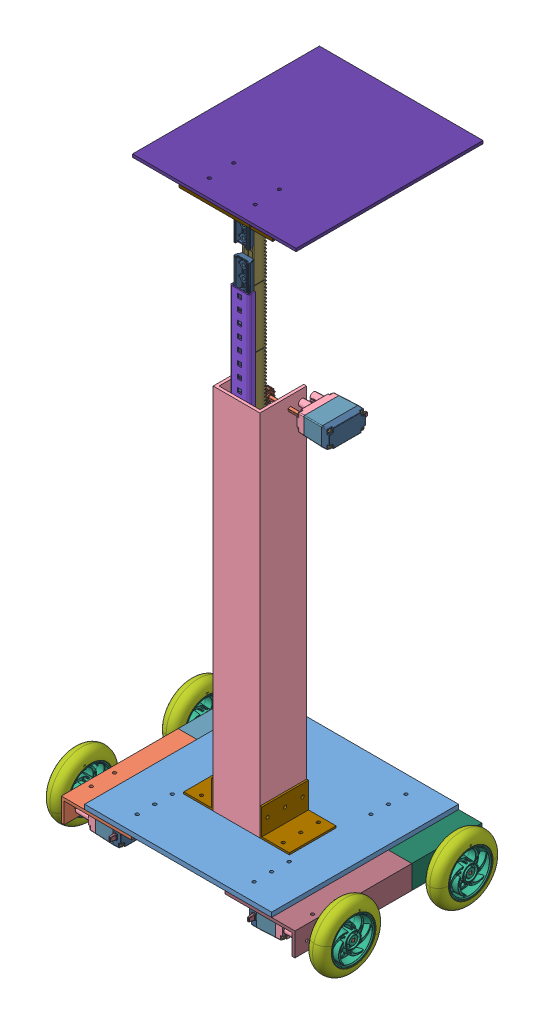
SolidWorks assembly mte380_Assy_01_lift_03., configuration Default. Lengths in mm.
Overall size (307.05 662.06 247.45).
139 component instances, 39 part files, 97 mates.
Components (placement in the parent):
- mte380_01_lift_base_02-1: mte380_01_lift_base_02 [Default] at (94.2351 110.2702 143.398) size (203.2 5 203.2)
- mte380_01_motor_bot_L_bracket_01-1: mte380_01_motor_bot_L_bracket_01 [Default] at (43.4351 110.2702 168.798) size (76.2 25.4 127)
- mte380_Assy_motor_vex_393_01-1: mte380_Assy_motor_vex_393_01 [Default] at (16.7501 95.0302 218.0279) x (0 0 -1) z (1 0 0) size (277.81 20.59 51.81)
  - SPPM206-0150BO-1: SPPM206-0150BO [Default] at (17.3 7.3 -1.5) x (1 0 0) z (0 -1 0) size (3.3 16.36 3.3)
  - 276-2181-003 Rev1-1: 276-2181-003 Rev1 [Default] at (0 0 -28) size (38.95 18.95 25.5)
  - 276-2177-019 Rev1-1: 276-2177-019 Rev1 [Default] at (-14.2702 0 -28) x (0.144195 -0.989549 0) z (0.989549 0.144195 0) size (6.3 15.8 6.3)
  - 276-2181-011 Rev1-1: 276-2181-011 Rev1 [Default] at (11.1298 0 -11) x (-1 0 0) z (0 1 0) size (11 4 11)
  - 276-2177-017 Rev1-1: 276-2177-017 Rev1 [Default] at (-245.51 0.1 2.5) size (248.21 15.59 2.54) (hidden)
  - QFK-N30QAV-16068-1: QFK-N30QAV-16068 [Default] at (-12.9 0 -23) x (0 1 0) z (0 0 1) size (12 10 26.1)
  - SPPM143-0030BO-1: SPPM143-0030BO [Default] at (-12.9 4.25 -6) x (-1 0 0) z (0 1 0) size (2.4 6.08 2.4)
  - 276-2181-010 Rev1-1: 276-2181-010 Rev1 [Default] at (10.8763 0 -9.4) x (0.878827 0.47714 0) z (0 0 1) size (1.5 1.5 16)
  - 276-2181-001 Rev1-1: 276-2181-001 Rev1 [Default] at origin size (40 20 8.01)
  - 276-2181-006 Rev1-1: 276-2181-006 Rev1 [Default] at (10.8763 0 -1.05) x (-0.259931 -0.965627 0) z (0 0 1) size (14.22 14.25 6.9)
  - 276-2181-007 Rev1-1: 276-2181-007 Rev1 [Default] at (2.1533 -1.4937 -4.4) x (-0.202497 0.979283 0) z (0 0 1) size (14.22 14.25 14.9)
  - 276-2181-010 Rev1-2: 276-2181-010 Rev1 [Default] at (-5.7003 2.586 -9.4) size (1.5 1.5 16)
  - 276-2177-018 Rev1-1: 276-2177-018 Rev1 [Default] at (-18.5 0.1 2.5) x (0 1 0) z (1 0 0) size (6.82 4.47 8.9)
  - 276-2181-006 Rev1-2: 276-2181-006 Rev1 [Default] at (2.1533 -1.4937 2.75) x (-0.071378 0.997449 0) z (0 0 1) size (14.22 14.25 6.9)
  - 276-2181-002 Rev1-1: 276-2181-002 Rev1 [Default] at (0 0 -20) size (40 20 23)
  - 276-2181-009 Rev1-1: 276-2181-009 Rev1 [Default] at (2.1533 -1.4937 -26.5) size (1.5 1.5 33)
  - SPPM206-0150BO-2: SPPM206-0150BO [Default] at (-16.9263 6.9263 -18.5) x (-0.075705 0.99713 0) z (-0.99713 -0.075705 0) size (3.3 16.36 3.3)
  - 276-2181-011 Rev1-2: 276-2181-011 Rev1 [Default] at (11.1298 0 -24) x (-0.997622 -0.068917 0) z (-0.068917 0.997622 0) size (11 4 11)
  - 276-2177-019 Rev1-2: 276-2177-019 Rev1 [Default] at (-1.5702 0 -28) x (0.32391 -0.946088 0) z (0.946088 0.32391 0) size (6.3 15.8 6.3)
  - SPPM206-0150BO-3: SPPM206-0150BO [Default] at (-17.3 -7.3 -1.5) x (0.292947 -0.956129 0) z (-0.956129 -0.292947 0) size (3.3 16.36 3.3)
  - SPPM206-0150BO-4: SPPM206-0150BO [Default] at (16.9263 -6.9263 -18.5) x (0.149257 -0.988799 0) z (0.988799 0.149257 0) size (3.3 16.36 3.3)
  - SPPM206-0150BO-5: SPPM206-0150BO [Default] at (17.3 -7.3 -1.5) x (1 0 0) z (0 -1 0) size (3.3 16.36 3.3)
  - SPPM206-0150BO-6: SPPM206-0150BO [Default] at (-16.9263 -6.9263 -18.5) x (-0.049887 0.998755 0) z (-0.998755 -0.049887 0) size (3.3 16.36 3.3)
  - SPPM206-0150BO-7: SPPM206-0150BO [Default] at (-17.3 7.3 -1.5) x (-0.963198 0.268794 0) z (0.268794 0.963198 0) size (3.3 16.36 3.3)
  - SPPM206-0150BO-8: SPPM206-0150BO [Default] at (16.9263 6.9263 -18.5) x (0.906825 0.421508 0) z (-0.421508 0.906825 0) size (3.3 16.36 3.3)
  - SPPM143-0030BO-2: SPPM143-0030BO [Default] at (-12.9 -4.25 -6) x (-0.988208 -0.153116 0) z (-0.153116 0.988208 0) size (2.4 6.08 2.4)
  - 276-2181-004 Rev1-1: 276-2181-004 Rev1 [Default] at (-12.9 0 -0.1) x (0.94341 -0.331628 0) z (0 0 -1) size (5.17 5.4 3)
  - 276-2181-005 Rev1-1: 276-2181-005 Rev1 [Default] at (-5.7003 2.586 -0.05) x (0.460478 -0.887671 0) z (0 0 1) size (11.88 11.88 5.9)
  - 276-2181-008 Rev1_276-2181-008g-1: 276-2181-008 Rev1_276-2181-008g [Default] at (11.1298 0 -14.5) x (0.267616 -0.963526 0) z (0 0 -1) size (13.83 13.88 17.3)
  - 276-2181-012 Rev1-1: 276-2181-012 Rev1 [Default] at (-12.9 0 -24) size (13.6 13 1)
- mte380_01_vex_shaft_2-1: mte380_01_vex_shaft_2 [Default] at (-31.9499 95.0479 206.9293) x (0 -0.267616 0.963526) z (-1 0 0) size (4.18 4.18 51.01)
- mte380_01_vex_bearing_block-1: mte380_01_vex_bearing_block [Default] at (-24.8662 107.0952 130.6495) x (0 0 -1) z (0 -1 0) size (35.56 10.16 13.39)
- mte380_01_center_shaft_01-1: mte380_01_center_shaft_01 [Default] at (68.8351 115.2702 130.698) size (50.8 400 50.8)
- mte380_Assy_wheel_vex_275-1: mte380_Assy_wheel_vex_275 [Default] at (-45.4869 83.9602 188.1506) x (0 0.267616 -0.963526) z (1 0 0) size (69.86 69.86 20.66)
  - SMALL-WHEEL-RIM-1: SMALL-WHEEL-RIM [Default] at (-15.1515 15.6838 -2.6601) size (61.43 61.43 9.24)
  - SMALL-WHEEL-HUB-1: SMALL-WHEEL-HUB [Default] at (-15.1515 15.6838 -2.6601) size (61.36 61.43 20.66)
  - SMALL-WHEEL-TIRE-1: SMALL-WHEEL-TIRE [Default] at (-15.1515 15.6838 -2.6601) x (1 0 0) z (0 -1 0) size (69.86 19.99 69.86)
- mte380_01_vex_rack_guide-1: mte380_01_vex_rack_guide [Default] at (94.2351 324.7702 178.323) x (-1 0 0) z (0 0 -1) size (20.84 444.5 8.8)
- mte380_01_vert_rack_bracket_01-1: mte380_01_vert_rack_bracket_01 [Default] at (119.6351 145.2702 130.698) size (32 30 50.8)
- mte380_01_vert_rack_bracket_01-2: mte380_01_vert_rack_bracket_01 [Default] at (68.8351 145.2702 181.498) x (-1 0 0) z (0 0 -1) size (32 30 50.8)
- mte380_01_vex_rack_slide-1: mte380_01_vex_rack_slide [Default] at (94.2351 619.0732 173.3216) x (1 0 0) z (0 1 0) size (17.45 8.37 50.79)
- mte380_01_vex_pinion_12-1: mte380_01_vex_pinion_12 [Default] at (93.6302 502.9979 149.2208) x (0 0.267616 -0.963526) z (1 0 0) size (14.8 14.8 9.53)
- mte380_01_vex_rack-1: mte380_01_vex_rack [Default] at (94.2351 650.8232 168.7501) x (0 1 0) z (-1 0 0) size (63 14.6 12.7)
- mte380_01_vex_rack_slide-2: mte380_01_vex_rack_slide [Default] at (94.2351 682.5732 173.3216) x (1 0 0) z (0 1 0) size (17.45 8.37 50.79)
- mte380_01_motor_bot_R_bracket_01-1: mte380_01_motor_bot_R_bracket_01 [Default] at (145.0351 110.2702 244.998) x (-1 0 0) z (0 0 -1) size (76.2 25.4 127)
- mte380_Assy_motor_vex_393_01-2: mte380_Assy_motor_vex_393_01 [Default] at (172.3201 95.0302 218.0279) x (0 0 -1) z (-1 0 0) size (277.81 20.59 51.81)
  - SPPM206-0150BO-1: SPPM206-0150BO [Default] at (17.3 7.3 -1.5) x (1 0 0) z (0 -1 0) size (3.3 16.36 3.3)
  - 276-2181-003 Rev1-1: 276-2181-003 Rev1 [Default] at (0 0 -28) size (38.95 18.95 25.5)
  - 276-2177-019 Rev1-1: 276-2177-019 Rev1 [Default] at (-14.2702 0 -28) x (0.144195 -0.989549 0) z (0.989549 0.144195 0) size (6.3 15.8 6.3)
  - 276-2181-011 Rev1-1: 276-2181-011 Rev1 [Default] at (11.1298 0 -11) x (-1 0 0) z (0 1 0) size (11 4 11)
  - 276-2177-017 Rev1-1: 276-2177-017 Rev1 [Default] at (-245.51 0.1 2.5) size (248.21 15.59 2.54) (hidden)
  - QFK-N30QAV-16068-1: QFK-N30QAV-16068 [Default] at (-12.9 0 -23) x (0 1 0) z (0 0 1) size (12 10 26.1)
  - SPPM143-0030BO-1: SPPM143-0030BO [Default] at (-12.9 4.25 -6) x (-1 0 0) z (0 1 0) size (2.4 6.08 2.4)
  - 276-2181-010 Rev1-1: 276-2181-010 Rev1 [Default] at (10.8763 0 -9.4) x (0.878827 0.47714 0) z (0 0 1) size (1.5 1.5 16)
  - 276-2181-001 Rev1-1: 276-2181-001 Rev1 [Default] at origin size (40 20 8.01)
  - 276-2181-006 Rev1-1: 276-2181-006 Rev1 [Default] at (10.8763 0 -1.05) x (-0.259931 -0.965627 0) z (0 0 1) size (14.22 14.25 6.9)
  - 276-2181-007 Rev1-1: 276-2181-007 Rev1 [Default] at (2.1533 -1.4937 -4.4) x (-0.202497 0.979283 0) z (0 0 1) size (14.22 14.25 14.9)
  - 276-2181-010 Rev1-2: 276-2181-010 Rev1 [Default] at (-5.7003 2.586 -9.4) size (1.5 1.5 16)
  - 276-2177-018 Rev1-1: 276-2177-018 Rev1 [Default] at (-18.5 0.1 2.5) x (0 1 0) z (1 0 0) size (6.82 4.47 8.9)
  - 276-2181-006 Rev1-2: 276-2181-006 Rev1 [Default] at (2.1533 -1.4937 2.75) x (-0.071378 0.997449 0) z (0 0 1) size (14.22 14.25 6.9)
  - 276-2181-002 Rev1-1: 276-2181-002 Rev1 [Default] at (0 0 -20) size (40 20 23)
  - 276-2181-009 Rev1-1: 276-2181-009 Rev1 [Default] at (2.1533 -1.4937 -26.5) size (1.5 1.5 33)
  - SPPM206-0150BO-2: SPPM206-0150BO [Default] at (-16.9263 6.9263 -18.5) x (-0.075705 0.99713 0) z (-0.99713 -0.075705 0) size (3.3 16.36 3.3)
  - 276-2181-011 Rev1-2: 276-2181-011 Rev1 [Default] at (11.1298 0 -24) x (-0.997622 -0.068917 0) z (-0.068917 0.997622 0) size (11 4 11)
  - 276-2177-019 Rev1-2: 276-2177-019 Rev1 [Default] at (-1.5702 0 -28) x (0.32391 -0.946088 0) z (0.946088 0.32391 0) size (6.3 15.8 6.3)
  - SPPM206-0150BO-3: SPPM206-0150BO [Default] at (-17.3 -7.3 -1.5) x (0.292947 -0.956129 0) z (-0.956129 -0.292947 0) size (3.3 16.36 3.3)
  - SPPM206-0150BO-4: SPPM206-0150BO [Default] at (16.9263 -6.9263 -18.5) x (0.149257 -0.988799 0) z (0.988799 0.149257 0) size (3.3 16.36 3.3)
  - SPPM206-0150BO-5: SPPM206-0150BO [Default] at (17.3 -7.3 -1.5) x (1 0 0) z (0 -1 0) size (3.3 16.36 3.3)
  - SPPM206-0150BO-6: SPPM206-0150BO [Default] at (-16.9263 -6.9263 -18.5) x (-0.049887 0.998755 0) z (-0.998755 -0.049887 0) size (3.3 16.36 3.3)
  - SPPM206-0150BO-7: SPPM206-0150BO [Default] at (-17.3 7.3 -1.5) x (-0.963198 0.268794 0) z (0.268794 0.963198 0) size (3.3 16.36 3.3)
  - SPPM206-0150BO-8: SPPM206-0150BO [Default] at (16.9263 6.9263 -18.5) x (0.906825 0.421508 0) z (-0.421508 0.906825 0) size (3.3 16.36 3.3)
  - SPPM143-0030BO-2: SPPM143-0030BO [Default] at (-12.9 -4.25 -6) x (-0.988208 -0.153116 0) z (-0.153116 0.988208 0) size (2.4 6.08 2.4)
  - 276-2181-004 Rev1-1: 276-2181-004 Rev1 [Default] at (-12.9 0 -0.1) x (0.94341 -0.331628 0) z (0 0 -1) size (5.17 5.4 3)
  - 276-2181-005 Rev1-1: 276-2181-005 Rev1 [Default] at (-5.7003 2.586 -0.05) x (0.460478 -0.887671 0) z (0 0 1) size (11.88 11.88 5.9)
  - 276-2181-008 Rev1_276-2181-008g-1: 276-2181-008 Rev1_276-2181-008g [Default] at (11.1298 0 -14.5) x (0.267616 -0.963526 0) z (0 0 -1) size (13.83 13.88 17.3)
  - 276-2181-012 Rev1-1: 276-2181-012 Rev1 [Default] at (-12.9 0 -24) size (13.6 13 1)
- mte380_01_vex_shaft_2-2: mte380_01_vex_shaft_2 [Default] at (221.0201 95.0615 206.9157) x (0 0.267616 0.963526) z (-1 0 0) size (4.18 4.18 51.01)
- mte380_Assy_wheel_vex_275-4: mte380_Assy_wheel_vex_275 [Default] at (239.8772 75.9124 196.4833) x (0 -0.267616 -0.963526) z (1 0 0) size (69.86 69.86 20.66)
  - SMALL-WHEEL-RIM-1: SMALL-WHEEL-RIM [Default] at (-15.1515 15.6838 -2.6601) size (61.43 61.43 9.24)
  - SMALL-WHEEL-HUB-1: SMALL-WHEEL-HUB [Default] at (-15.1515 15.6838 -2.6601) size (61.36 61.43 20.66)
  - SMALL-WHEEL-TIRE-1: SMALL-WHEEL-TIRE [Default] at (-15.1515 15.6838 -2.6601) x (1 0 0) z (0 -1 0) size (69.86 19.99 69.86)
- mte380_01_vex_shaft_2-3: mte380_01_vex_shaft_2 [Default] at (221.2351 95.0937 79.8345) x (0 0 1) z (-1 0 0) size (4.18 4.18 51.01)
- mte380_01_vex_shaft_2-4: mte380_01_vex_shaft_2 [Default] at (-32.7649 95.1912 79.8345) x (0 0 1) z (-1 0 0) size (4.18 4.18 51.01)
- mte380_01_front_bot_L_bracket_01-1: mte380_01_front_bot_L_bracket_01 [Default] at (43.4351 110.2702 41.798) size (76.2 25.4 76.2)
- mte380_01_front_bot_R_bracket_01-1: mte380_01_front_bot_R_bracket_01 [Default] at (145.0351 110.2702 117.998) x (-1 0 0) z (0 0 -1) size (76.2 25.4 76.2)
- mte380_01_vex_flat_bearing-2: mte380_01_vex_flat_bearing [Default] at (129.0839 107.7302 106.314) x (1 0 0) z (0 1 0) size (7.04 35.56 10.16)
- mte380_01_vex_flat_bearing-3: mte380_01_vex_flat_bearing [Default] at (59.3863 107.7302 53.482) x (-1 0 0) z (0 1 0) size (7.04 35.56 10.16)
- mte380_Assy_wheel_vex_275-5: mte380_Assy_wheel_vex_275 [Default] at (-46.3019 79.4824 64.708) x (0 0 -1) z (1 0 0) size (69.86 69.86 20.66)
  - SMALL-WHEEL-RIM-1: SMALL-WHEEL-RIM [Default] at (-15.1515 15.6838 -2.6601) size (61.43 61.43 9.24)
  - SMALL-WHEEL-HUB-1: SMALL-WHEEL-HUB [Default] at (-15.1515 15.6838 -2.6601) size (61.36 61.43 20.66)
  - SMALL-WHEEL-TIRE-1: SMALL-WHEEL-TIRE [Default] at (-15.1515 15.6838 -2.6601) x (1 0 0) z (0 -1 0) size (69.86 19.99 69.86)
- mte380_Assy_wheel_vex_275-6: mte380_Assy_wheel_vex_275 [Default] at (240.0922 79.4349 64.658) x (0 0 -1) z (1 0 0) size (69.86 69.86 20.66)
  - SMALL-WHEEL-RIM-1: SMALL-WHEEL-RIM [Default] at (-15.1515 15.6838 -2.6601) size (61.43 61.43 9.24)
  - SMALL-WHEEL-HUB-1: SMALL-WHEEL-HUB [Default] at (-15.1515 15.6838 -2.6601) size (61.36 61.43 20.66)
  - SMALL-WHEEL-TIRE-1: SMALL-WHEEL-TIRE [Default] at (-15.1515 15.6838 -2.6601) x (1 0 0) z (0 -1 0) size (69.86 19.99 69.86)
- mte380_Assy_motor_vex_393_01-3: mte380_Assy_motor_vex_393_01 [Default] at (163.3228 503.011 138.0423) x (0 0 1) z (1 0 0) size (277.81 20.59 51.81)
  - SPPM206-0150BO-1: SPPM206-0150BO [Default] at (17.3 7.3 -1.5) x (1 0 0) z (0 -1 0) size (3.3 16.36 3.3)
  - 276-2181-003 Rev1-1: 276-2181-003 Rev1 [Default] at (0 0 -28) size (38.95 18.95 25.5)
  - 276-2177-019 Rev1-1: 276-2177-019 Rev1 [Default] at (-14.2702 0 -28) x (0.144195 -0.989549 0) z (0.989549 0.144195 0) size (6.3 15.8 6.3)
  - 276-2181-011 Rev1-1: 276-2181-011 Rev1 [Default] at (11.1298 0 -11) x (-1 0 0) z (0 1 0) size (11 4 11)
  - 276-2177-017 Rev1-1: 276-2177-017 Rev1 [Default] at (-245.51 0.1 2.5) size (248.21 15.59 2.54) (hidden)
  - QFK-N30QAV-16068-1: QFK-N30QAV-16068 [Default] at (-12.9 0 -23) x (0 1 0) z (0 0 1) size (12 10 26.1)
  - SPPM143-0030BO-1: SPPM143-0030BO [Default] at (-12.9 4.25 -6) x (-1 0 0) z (0 1 0) size (2.4 6.08 2.4)
  - 276-2181-010 Rev1-1: 276-2181-010 Rev1 [Default] at (10.8763 0 -9.4) x (0.878827 0.47714 0) z (0 0 1) size (1.5 1.5 16)
  - 276-2181-001 Rev1-1: 276-2181-001 Rev1 [Default] at origin size (40 20 8.01)
  - 276-2181-006 Rev1-1: 276-2181-006 Rev1 [Default] at (10.8763 0 -1.05) x (-0.259931 -0.965627 0) z (0 0 1) size (14.22 14.25 6.9)
  - 276-2181-007 Rev1-1: 276-2181-007 Rev1 [Default] at (2.1533 -1.4937 -4.4) x (-0.202497 0.979283 0) z (0 0 1) size (14.22 14.25 14.9)
  - 276-2181-010 Rev1-2: 276-2181-010 Rev1 [Default] at (-5.7003 2.586 -9.4) size (1.5 1.5 16)
  - 276-2177-018 Rev1-1: 276-2177-018 Rev1 [Default] at (-18.5 0.1 2.5) x (0 1 0) z (1 0 0) size (6.82 4.47 8.9)
  - 276-2181-006 Rev1-2: 276-2181-006 Rev1 [Default] at (2.1533 -1.4937 2.75) x (-0.071378 0.997449 0) z (0 0 1) size (14.22 14.25 6.9)
  - 276-2181-002 Rev1-1: 276-2181-002 Rev1 [Default] at (0 0 -20) size (40 20 23)
  - 276-2181-009 Rev1-1: 276-2181-009 Rev1 [Default] at (2.1533 -1.4937 -26.5) size (1.5 1.5 33)
  - SPPM206-0150BO-2: SPPM206-0150BO [Default] at (-16.9263 6.9263 -18.5) x (-0.075705 0.99713 0) z (-0.99713 -0.075705 0) size (3.3 16.36 3.3)
  - 276-2181-011 Rev1-2: 276-2181-011 Rev1 [Default] at (11.1298 0 -24) x (-0.997622 -0.068917 0) z (-0.068917 0.997622 0) size (11 4 11)
  - 276-2177-019 Rev1-2: 276-2177-019 Rev1 [Default] at (-1.5702 0 -28) x (0.32391 -0.946088 0) z (0.946088 0.32391 0) size (6.3 15.8 6.3)
  - SPPM206-0150BO-3: SPPM206-0150BO [Default] at (-17.3 -7.3 -1.5) x (0.292947 -0.956129 0) z (-0.956129 -0.292947 0) size (3.3 16.36 3.3)
  - SPPM206-0150BO-4: SPPM206-0150BO [Default] at (16.9263 -6.9263 -18.5) x (0.149257 -0.988799 0) z (0.988799 0.149257 0) size (3.3 16.36 3.3)
  - SPPM206-0150BO-5: SPPM206-0150BO [Default] at (17.3 -7.3 -1.5) x (1 0 0) z (0 -1 0) size (3.3 16.36 3.3)
  - SPPM206-0150BO-6: SPPM206-0150BO [Default] at (-16.9263 -6.9263 -18.5) x (-0.049887 0.998755 0) z (-0.998755 -0.049887 0) size (3.3 16.36 3.3)
  - SPPM206-0150BO-7: SPPM206-0150BO [Default] at (-17.3 7.3 -1.5) x (-0.963198 0.268794 0) z (0.268794 0.963198 0) size (3.3 16.36 3.3)
  - SPPM206-0150BO-8: SPPM206-0150BO [Default] at (16.9263 6.9263 -18.5) x (0.906825 0.421508 0) z (-0.421508 0.906825 0) size (3.3 16.36 3.3)
  - SPPM143-0030BO-2: SPPM143-0030BO [Default] at (-12.9 -4.25 -6) x (-0.988208 -0.153116 0) z (-0.153116 0.988208 0) size (2.4 6.08 2.4)
  - 276-2181-004 Rev1-1: 276-2181-004 Rev1 [Default] at (-12.9 0 -0.1) x (0.94341 -0.331628 0) z (0 0 -1) size (5.17 5.4 3)
  - 276-2181-005 Rev1-1: 276-2181-005 Rev1 [Default] at (-5.7003 2.586 -0.05) x (0.460478 -0.887671 0) z (0 0 1) size (11.88 11.88 5.9)
  - 276-2181-008 Rev1_276-2181-008g-1: 276-2181-008 Rev1_276-2181-008g [Default] at (11.1298 0 -14.5) x (0.267616 -0.963526 0) z (0 0 -1) size (13.83 13.88 17.3)
  - 276-2181-012 Rev1-1: 276-2181-012 Rev1 [Default] at (-12.9 0 -24) size (13.6 13 1)
- mte380_01_vex_shaft_2-5: mte380_01_vex_shaft_2 [Default] at (114.6228 503.0287 149.2034) x (0 -0.267616 0.963526) z (-1 0 0) size (4.18 4.18 51.01)
- mte380_01_lift_platform_02-1: mte380_01_lift_platform_02 [Default] at (183.1351 710.8982 2.498) size (177.8 3.17 203.2)
- mte380_01_lift_platform__bracket_01-1: mte380_01_lift_platform__bracket_01 [Default] at (132.3351 682.3232 168.7501) x (0 0 1) z (-1 0 0) size (28.57 28.57 76.2)
- mte380_01_lift_platform__bracket_01-2: mte380_01_lift_platform__bracket_01 [Default] at (56.1351 682.3232 177.123) x (0 0 -1) z (1 0 0) size (28.57 28.57 76.2)
- mte380_01_vex_rack_slide-3: mte380_01_vex_rack_slide [Default] at (94.2351 492.0732 173.3216) x (1 0 0) z (0 1 0) size (17.45 8.37 50.79)
- mte380_01_vex_rack-2: mte380_01_vex_rack [Default] at (94.2351 523.8232 168.7501) x (0 1 0) z (-1 0 0) size (63 14.6 12.7)
- mte380_01_vex_rack_slide-4: mte380_01_vex_rack_slide [Default] at (94.2351 555.5732 173.3216) x (1 0 0) z (0 1 0) size (17.45 8.37 50.79)
- mte380_01_vex_rack-3: mte380_01_vex_rack [Default] at (94.2351 587.3232 168.7501) x (0 1 0) z (-1 0 0) size (63 14.6 12.7)
- Part2^mte380_Assy_01_lift_03.-1: Part2^mte380_Assy_01_lift_03. [Default] at (43.4351 110.2702 41.798) x (1 0 0) z (0 1 0) (virtual)
- mte380_01_lift_base_support_bracket_01-1: mte380_01_lift_base_support_bracket_01 [Default] at (145.0351 110.2702 92.598) x (-1 0 0) z (0 0 1) size (101.6 25.4 50.8)
Mates (geometry in assembly coordinates):
- Coincident2: coincident: line of mte380_01_lift_base_02-1 through (-7.3649 110.2702 244.998) axis (1 0 0); plane of mte380_01_motor_bot_L_bracket_01-1 through (43.4351 110.2702 244.998) normal (0 0 1)
- Coincident7: coincident anti-aligned: plane of mte380_Assy_motor_vex_393_01-1/276-2181-008 Rev1_276-2181-008g-1 through (-6.5499 96.1526 208.8837) normal (0 0.267616 -0.963526); plane of mte380_01_vex_shaft_2-1 through (-57.3499 93.0935 208.034) normal (0 -0.267616 0.963526)
- Coincident8: coincident anti-aligned: plane of mte380_Assy_motor_vex_393_01-1/276-2181-008 Rev1_276-2181-008g-1 through (-6.5499 97.0159 205.7756) normal (0 -0.963526 -0.267616); plane of mte380_01_vex_shaft_2-1 through (-57.3499 97.0023 205.8245) normal (0 0.963526 0.267616)
- Coincident9: coincident anti-aligned: plane of mte380_Assy_motor_vex_393_01-1/276-2181-008 Rev1_276-2181-008g-1 through (-6.5499 93.0445 208.0204) normal (-1 0 0); plane of mte380_01_vex_shaft_2-1 through (-6.5499 97.0023 205.8245) normal (1 0 0)
- Coincident10: coincident anti-aligned: plane of mte380_01_lift_base_02-1 through (94.2351 110.2702 143.398) normal (0 -1 0); plane of mte380_01_motor_bot_L_bracket_01-1 through (43.4351 110.2702 244.998) normal (0 1 0)
- Coincident29: coincident aligned: plane of mte380_01_lift_base_02-1 through (-7.3649 115.2702 244.998) normal (0 0 1); plane of mte380_01_motor_bot_L_bracket_01-1 through (43.4351 110.2702 244.998) normal (0 0 1)
- Distance3: distance = 50.8 mm anti-aligned: plane of mte380_01_lift_base_02-1 through (-7.3649 115.2702 244.998) normal (-1 0 0); plane of mte380_01_motor_bot_L_bracket_01-1 through (43.4351 107.0952 244.998) normal (1 0 0)
- Distance5: distance = 2.54 mm anti-aligned: plane of mte380_Assy_motor_vex_393_01-1/276-2177-019 Rev1-2 through (-27.0499 95.0302 219.598) normal (-1 0 0); plane of mte380_01_motor_bot_L_bracket_01-1 through (-29.5899 84.8702 244.998) normal (1 0 0)
- Coincident48: coincident anti-aligned: plane of mte380_01_lift_base_02-1 through (94.2351 115.2702 143.398) normal (0 1 0); plane of mte380_01_center_shaft_01-1 through (68.8351 115.2702 130.698) normal (0 -1 0)
- Width1: width anti-aligned: plane of mte380_01_lift_base_02-1 through (-7.3649 115.2702 244.998) normal (-1 0 0); plane of mte380_01_lift_base_02-1 through (195.8351 115.2702 244.998) normal (1 0 0); plane of mte380_01_center_shaft_01-1 through (119.6351 515.2702 181.498) normal (1 0 0); plane of mte380_01_center_shaft_01-1 through (68.8351 515.2702 130.698) normal (-1 0 0)
- Distance6: distance = 63.5 mm aligned: plane of mte380_01_center_shaft_01-1 through (68.8351 515.2702 181.498) normal (0 0 1); plane of mte380_01_lift_base_02-1 through (-7.3649 115.2702 244.998) normal (0 0 1)
- Coincident52: coincident anti-aligned: plane of mte380_01_vex_shaft_2-1 through (-57.3499 93.9431 204.9748) normal (0 0.267616 -0.963526); plane of mte380_Assy_wheel_vex_275-1/SMALL-WHEEL-HUB-1 through (-36.717 93.895 204.9615) normal (0 -0.267616 0.963526)
- Coincident53: coincident anti-aligned: plane of mte380_01_vex_shaft_2-1 through (-57.3499 97.0023 205.8245) normal (0 0.963526 0.267616); plane of mte380_Assy_wheel_vex_275-1/SMALL-WHEEL-HUB-1 through (-36.717 97.0023 205.8245) normal (0 -0.963526 -0.267616)
- Tangent9: tangent anti-aligned: plane of mte380_01_vex_shaft_2-1 through (-57.3499 97.0023 205.8245) normal (-1 0 0); sphere of mte380_Assy_wheel_vex_275-1/SMALL-WHEEL-HUB-1
- Coincident55: coincident anti-aligned: plane of mte380_01_center_shaft_01-1 through (116.4601 515.2702 178.323) normal (0 0 -1); plane of mte380_01_vex_rack_guide-1 through (85.7693 172.3702 178.323) normal (0 0 1)
- Width2: width anti-aligned: plane of mte380_01_center_shaft_01-1 through (116.4601 515.2702 130.698) normal (-1 0 0); plane of mte380_01_center_shaft_01-1 through (72.0101 515.2702 178.323) normal (1 0 0); plane of mte380_01_vex_rack_guide-1 through (104.59 172.3702 175.861) normal (0.965926 0 -0.258819); plane of mte380_01_vex_rack_guide-1 through (85.5782 172.3702 169.5238) normal (-0.965926 0 -0.258819)
- Coincident56: coincident anti-aligned: plane of mte380_01_center_shaft_01-1 through (119.6351 515.2702 181.498) normal (1 0 0); plane of mte380_01_vert_rack_bracket_01-1 through (119.6351 145.2702 181.498) normal (-1 0 0)
- Coincident57: coincident anti-aligned: plane of mte380_01_lift_base_02-1 through (94.2351 115.2702 143.398) normal (0 1 0); plane of mte380_01_vert_rack_bracket_01-1 through (119.6351 115.2702 181.498) normal (0 -1 0)
- Coincident58: coincident anti-aligned: plane of mte380_01_center_shaft_01-1 through (68.8351 515.2702 130.698) normal (-1 0 0); plane of mte380_01_vert_rack_bracket_01-2 through (68.8351 145.2702 130.698) normal (1 0 0)
- Coincident59: coincident anti-aligned: plane of mte380_01_lift_base_02-1 through (94.2351 115.2702 143.398) normal (0 1 0); plane of mte380_01_vert_rack_bracket_01-2 through (68.8351 115.2702 130.698) normal (0 -1 0)
- Coincident61: coincident anti-aligned: plane of mte380_01_vex_rack_guide-1 through (102.7008 172.3702 177.123) normal (0 0 -1); plane of mte380_01_vex_rack_slide-1 through (94.2351 619.0732 177.123) normal (0 0 1)
- Width3: width anti-aligned: plane of mte380_01_vex_rack_slide-1 through (103.5283 644.4732 177.2489) normal (0.965926 0 -0.258819); plane of mte380_01_vex_rack_slide-1 through (87.0326 644.4732 169.446) normal (-0.965926 0 -0.258819); plane of mte380_01_vex_rack_guide-1 through (101.7328 172.3702 169.8344) normal (-0.965926 0 0.258819); plane of mte380_01_vex_rack_guide-1 through (85.0393 172.3702 176.1716) normal (0.965926 0 0.258819)
- Coincident63: coincident anti-aligned: plane of mte380_01_vex_rack_slide-1 through (101.5342 644.4732 168.7501) normal (0 0 -1); plane of mte380_01_vex_rack-1 through (94.2351 650.8232 168.7501) normal (0 0 1)
- Coincident64: coincident anti-aligned: plane of mte380_01_vex_rack_guide-1 through (102.7008 172.3702 177.123) normal (0 0 -1); plane of mte380_01_vex_rack_slide-2 through (94.2351 682.5732 177.123) normal (0 0 1)
- Width4: width anti-aligned: plane of mte380_01_vex_rack_slide-2 through (103.5283 707.9732 177.2489) normal (0.965926 0 -0.258819); plane of mte380_01_vex_rack_slide-2 through (87.0326 707.9732 169.446) normal (-0.965926 0 -0.258819); plane of mte380_01_vex_rack_guide-1 through (101.7328 172.3702 169.8344) normal (-0.965926 0 0.258819); plane of mte380_01_vex_rack_guide-1 through (85.0393 172.3702 176.1716) normal (0.965926 0 0.258819)
- Concentric9: concentric anti-aligned: cylinder of mte380_01_vex_rack_slide-1 through (94.2351 625.4232 168.7501) axis (0 0 -1) radius 1.85; cylinder of mte380_01_vex_rack-1 through (94.2351 625.4232 168.7501) axis (0 0 1) radius 2.25
- Concentric12: concentric anti-aligned: cylinder of mte380_01_vex_rack-1 through (94.2351 676.2232 168.7501) axis (0 0 1) radius 2.25; cylinder of mte380_01_vex_rack_slide-2 through (94.2351 676.2232 168.7501) axis (0 0 -1) radius 1.85
- Coincident65: coincident aligned: plane of mte380_01_center_shaft_01-1 through (119.6351 515.2702 130.698) normal (0 0 -1); plane of mte380_01_vert_rack_bracket_01-1 through (119.6351 145.2702 130.698) normal (0 0 -1)
- Coincident66: coincident aligned: plane of mte380_01_center_shaft_01-1 through (72.0101 515.2702 130.698) normal (0 0 -1); plane of mte380_01_vert_rack_bracket_01-2 through (68.8351 145.2702 130.698) normal (0 0 -1)
- Coincident67: coincident anti-aligned: plane of mte380_01_lift_base_02-1 through (94.2351 110.2702 143.398) normal (0 -1 0); plane of mte380_01_motor_bot_R_bracket_01-1 through (145.0351 110.2702 168.798) normal (0 1 0)
- Coincident68: coincident aligned: plane of mte380_01_lift_base_02-1 through (-7.3649 115.2702 244.998) normal (0 0 1); plane of mte380_01_motor_bot_R_bracket_01-1 through (145.0351 110.2702 244.998) normal (0 0 1)
- Distance7: distance = 50.8 mm: line of mte380_01_lift_base_02-1 through (195.8351 115.2702 244.998) axis (0 -1 0); line of mte380_01_motor_bot_R_bracket_01-1 through (145.0351 107.0952 244.998) axis (0 1 0)
- Concentric13: concentric aligned: cylinder of mte380_01_motor_bot_R_bracket_01-1 through (221.2351 95.0302 219.598) axis (1 0 0) radius 1.3526; cylinder of mte380_Assy_motor_vex_393_01-2/276-2177-019 Rev1-2 through (216.1201 95.0302 219.598) axis (1 0 0) radius 1.3526
- Concentric14: concentric aligned: cylinder of mte380_01_motor_bot_R_bracket_01-1 through (221.2351 95.0302 232.298) axis (1 0 0) radius 1.3526; cylinder of mte380_Assy_motor_vex_393_01-2/276-2177-019 Rev1-1 through (216.1201 95.0302 232.298) axis (1 0 0) radius 1.3526
- Distance8: distance = 2.54 mm anti-aligned: plane of mte380_Assy_motor_vex_393_01-2/276-2181-003 Rev1-1 through (215.5201 95.0302 218.0279) normal (1 0 0); plane of mte380_01_motor_bot_R_bracket_01-1 through (218.0601 84.8702 168.798) normal (-1 0 0)
- Coincident71: coincident anti-aligned: plane of mte380_Assy_motor_vex_393_01-2/276-2181-008 Rev1_276-2181-008g-1 through (195.6201 97.0159 208.0204) normal (1 0 0); plane of mte380_01_vex_shaft_2-2 through (195.6201 96.1662 204.9613) normal (-1 0 0)
- Coincident72: coincident anti-aligned: plane of mte380_Assy_motor_vex_393_01-2/276-2181-008 Rev1_276-2181-008g-1 through (195.6201 96.1526 204.9123) normal (0 -0.963526 0.267616); plane of mte380_01_vex_shaft_2-2 through (195.6201 96.1662 204.9613) normal (0 0.963526 -0.267616)
- Coincident73: coincident anti-aligned: plane of mte380_Assy_motor_vex_393_01-2/276-2181-008 Rev1_276-2181-008g-1 through (195.6201 93.9078 208.8837) normal (0 -0.267616 -0.963526); plane of mte380_01_vex_shaft_2-2 through (195.6201 93.9567 208.8701) normal (0 0.267616 0.963526)
- Coincident74: coincident anti-aligned: plane of mte380_01_vex_shaft_2-2 through (195.6201 93.107 205.8109) normal (0 -0.963526 0.267616); plane of mte380_Assy_wheel_vex_275-4/SMALL-WHEEL-HUB-1 through (248.6472 93.9567 208.8701) normal (0 0.963526 -0.267616)
- Coincident76: coincident anti-aligned: plane of mte380_01_vex_shaft_2-2 through (195.6201 93.9567 208.8701) normal (0 0.267616 0.963526); plane of mte380_Assy_wheel_vex_275-4/SMALL-WHEEL-HUB-1 through (248.6472 97.0641 208.0071) normal (0 -0.267616 -0.963526)
- Tangent11: tangent anti-aligned: plane of mte380_01_vex_shaft_2-2 through (246.4201 96.1662 204.9613) normal (1 0 0); sphere of mte380_Assy_wheel_vex_275-4/SMALL-WHEEL-HUB-1
- Concentric17: concentric anti-aligned: cylinder of mte380_01_motor_bot_L_bracket_01-1 through (-25.5934 110.2702 219.598) axis (0 1 0) radius 1.7272; cone of mte380_01_vex_bearing_block-1 through (-25.5934 107.0952 219.598) axis (0 -1 0)
- Distance13: distance = 0 mm anti-aligned: plane of mte380_01_vex_bearing_block-1 through (-31.6896 107.0952 228.2341) normal (0 1 0); plane of mte380_01_motor_bot_L_bracket_01-1 through (-29.5899 107.0952 244.998) normal (0 -1 0)
- Concentric18: concentric aligned: cylinder of mte380_01_motor_bot_L_bracket_01-1 through (-32.7649 95.0302 232.298) axis (-1 0 0) radius 1.3526; circle of mte380_Assy_motor_vex_393_01-1/276-2177-019 Rev1-1
- Concentric19: concentric aligned: circle of mte380_01_motor_bot_L_bracket_01-1; circle of mte380_Assy_motor_vex_393_01-1/276-2177-019 Rev1-2
- Coincident99: coincident anti-aligned: plane of mte380_01_lift_base_02-1 through (94.2351 110.2702 143.398) normal (0 -1 0); plane of mte380_01_front_bot_L_bracket_01-1 through (43.4351 110.2702 117.998) normal (0 1 0)
- Coincident100: coincident aligned: plane of mte380_01_lift_base_02-1 through (-7.3649 115.2702 41.798) normal (0 0 -1); plane of mte380_01_front_bot_L_bracket_01-1 through (43.4351 110.2702 41.798) normal (0 0 -1)
- Distance14: distance = 50.8 mm anti-aligned: plane of mte380_01_front_bot_L_bracket_01-1 through (43.4351 107.0952 117.998) normal (1 0 0); plane of mte380_01_lift_base_02-1 through (-7.3649 115.2702 244.998) normal (-1 0 0)
- Coincident102: coincident anti-aligned: plane of mte380_01_lift_base_02-1 through (94.2351 110.2702 143.398) normal (0 -1 0); plane of mte380_01_front_bot_R_bracket_01-1 through (145.0351 110.2702 41.798) normal (0 1 0)
- Coincident103: coincident aligned: plane of mte380_01_lift_base_02-1 through (-7.3649 115.2702 41.798) normal (0 0 -1); plane of mte380_01_front_bot_R_bracket_01-1 through (145.0351 110.2702 41.798) normal (0 0 -1)
- Distance16: distance = 50.8 mm anti-aligned: plane of mte380_01_front_bot_R_bracket_01-1 through (145.0351 107.0952 41.798) normal (-1 0 0); plane of mte380_01_lift_base_02-1 through (195.8351 115.2702 244.998) normal (1 0 0)
- Concentric20: concentric anti-aligned: cylinder of mte380_01_front_bot_R_bracket_01-1 through (221.2351 95.0302 67.198) axis (1 0 0) radius 1.7272; circle of mte380_01_vex_flat_bearing-2
- Coincident106: coincident anti-aligned: plane of mte380_01_front_bot_R_bracket_01-1 through (218.0601 84.8702 41.798) normal (-1 0 0); plane of mte380_01_vex_flat_bearing-2 through (218.0601 107.7302 106.314) normal (1 0 0)
- Concentric21: concentric anti-aligned: circle of mte380_01_front_bot_R_bracket_01-1; cylinder of mte380_01_vex_flat_bearing-2 through (211.7101 95.0302 92.598) axis (-1 0 0) radius 2.1209
- Concentric22: concentric anti-aligned: cylinder of mte380_01_front_bot_L_bracket_01-1 through (-32.7649 95.0302 67.198) axis (-1 0 0) radius 1.7272; cylinder of mte380_01_vex_flat_bearing-3 through (-23.2399 95.0302 67.198) axis (1 0 0) radius 2.1209
- Concentric23: concentric anti-aligned: cylinder of mte380_01_front_bot_L_bracket_01-1 through (-32.7649 95.0302 92.598) axis (-1 0 0) radius 1.7272; cylinder of mte380_01_vex_flat_bearing-3 through (-23.2399 95.0302 92.598) axis (1 0 0) radius 2.1209
- Coincident107: coincident anti-aligned: plane of mte380_01_front_bot_L_bracket_01-1 through (-29.5899 84.8702 117.998) normal (1 0 0); plane of mte380_01_vex_flat_bearing-3 through (-29.5899 107.7302 53.482) normal (-1 0 0)
- Coincident108: coincident anti-aligned: plane of mte380_01_vex_shaft_2-4 through (-58.1649 93.6037 78.247) normal (0 0 -1); plane of mte380_Assy_wheel_vex_275-5/SMALL-WHEEL-HUB-1 through (-37.532 93.5537 78.247) normal (0 0 1)
- Coincident109: coincident anti-aligned: plane of mte380_01_vex_shaft_2-4 through (-58.1649 96.7787 78.247) normal (0 1 0); plane of mte380_Assy_wheel_vex_275-5/SMALL-WHEEL-HUB-1 through (-37.532 96.7787 78.247) normal (0 -1 0)
- Tangent12: tangent anti-aligned: plane of mte380_01_vex_shaft_2-4 through (-58.1649 96.7787 78.247) normal (-1 0 0); sphere of mte380_Assy_wheel_vex_275-5/SMALL-WHEEL-HUB-1
- Coincident110: coincident anti-aligned: plane of mte380_01_vex_shaft_2-3 through (195.8351 93.5062 81.422) normal (0 0 1); plane of mte380_Assy_wheel_vex_275-6/SMALL-WHEEL-HUB-1 through (248.8622 96.7312 81.422) normal (0 0 -1)
- Coincident111: coincident anti-aligned: plane of mte380_01_vex_shaft_2-3 through (195.8351 93.5062 78.247) normal (0 -1 0); plane of mte380_Assy_wheel_vex_275-6/SMALL-WHEEL-HUB-1 through (248.8622 93.5062 81.422) normal (0 1 0)
- Tangent13: tangent anti-aligned: plane of mte380_01_vex_shaft_2-3 through (246.6351 96.6812 78.247) normal (1 0 0); sphere of mte380_Assy_wheel_vex_275-6/SMALL-WHEEL-HUB-1
- Coincident125: coincident anti-aligned: plane of mte380_Assy_motor_vex_393_01-3/276-2181-008 Rev1_276-2181-008g-1 through (140.0228 504.1334 151.1578) normal (0 -0.963526 -0.267616); plane of mte380_01_vex_shaft_2-5 through (89.2228 504.9831 148.0986) normal (0 0.963526 0.267616)
- Coincident126: coincident anti-aligned: plane of mte380_Assy_motor_vex_393_01-3/276-2181-008 Rev1_276-2181-008g-1 through (140.0228 501.0253 150.2945) normal (0 0.267616 -0.963526); plane of mte380_01_vex_shaft_2-5 through (89.2228 501.0742 150.3081) normal (0 -0.267616 0.963526)
- Coincident127: coincident anti-aligned: plane of mte380_Assy_motor_vex_393_01-3/276-2181-008 Rev1_276-2181-008g-1 through (140.0228 504.9967 148.0497) normal (-1 0 0); plane of mte380_01_vex_shaft_2-5 through (140.0228 504.9831 148.0986) normal (1 0 0)
- Coincident129: coincident anti-aligned: plane of mte380_01_vex_pinion_12-1 through (98.3927 504.3468 147.9219) normal (0 -0.267616 0.963526); plane of mte380_01_vex_shaft_2-5 through (89.2228 501.9239 147.2489) normal (0 0.267616 -0.963526)
- Coincident130: coincident anti-aligned: plane of mte380_01_vex_pinion_12-1 through (98.3927 504.2968 150.5697) normal (0 -0.963526 -0.267616); plane of mte380_01_vex_shaft_2-5 through (89.2228 504.9831 148.0986) normal (0 0.963526 0.267616)
- Distance17: distance = 101.6 mm aligned: plane of mte380_01_vex_rack_guide-1 through (85.7693 616.8702 176.3672) normal (0 1 0); plane of mte380_01_center_shaft_01-1 through (68.8351 515.2702 130.698) normal (0 1 0)
- Coincident135: coincident anti-aligned: plane of mte380_01_vex_rack_slide-2 through (101.5342 707.9732 168.7501) normal (0 0 -1); plane of mte380_01_lift_platform__bracket_01-1 through (56.1351 682.3232 168.7501) normal (0 0 1)
- Width6: width anti-aligned: plane of mte380_01_vex_rack_slide-2 through (87.5934 707.9732 169.4201) normal (-0.965926 0 -0.258819); plane of mte380_01_vex_rack_slide-2 through (100.8768 707.9732 169.4201) normal (0.965926 0 -0.258819); plane of mte380_01_lift_platform__bracket_01-1 through (132.3351 682.3232 168.7501) normal (1 0 0); plane of mte380_01_lift_platform__bracket_01-1 through (56.1351 682.3232 168.7501) normal (-1 0 0)
- Coincident136: coincident anti-aligned: plane of mte380_01_vex_rack-1 through (87.8851 682.3232 93.3328) normal (0 1 0); plane of mte380_01_lift_platform__bracket_01-1 through (56.1351 682.3232 165.5751) normal (0 -1 0)
- Coincident137: coincident anti-aligned: plane of mte380_01_vex_rack_slide-2 through (94.2351 682.5732 177.123) normal (0 0 1); plane of mte380_01_lift_platform__bracket_01-2 through (132.3351 682.3232 177.123) normal (0 0 -1)
- Coincident138: coincident aligned: plane of mte380_01_lift_platform__bracket_01-1 through (56.1351 710.8982 168.7501) normal (0 1 0); plane of mte380_01_lift_platform__bracket_01-2 through (132.3351 710.8982 177.123) normal (0 1 0)
- Width7: width anti-aligned: plane of mte380_01_vex_rack_slide-2 through (87.0326 707.9732 169.446) normal (-0.965926 0 -0.258819); plane of mte380_01_vex_rack_slide-2 through (103.5283 707.9732 177.2489) normal (0.965926 0 -0.258819); plane of mte380_01_lift_platform__bracket_01-2 through (132.3351 682.3232 177.123) normal (1 0 0); plane of mte380_01_lift_platform__bracket_01-2 through (56.1351 682.3232 177.123) normal (-1 0 0)
- Coincident139: coincident anti-aligned: plane of mte380_01_lift_platform_02-1 through (183.1351 710.8982 2.498) normal (0 -1 0); plane of mte380_01_lift_platform__bracket_01-1 through (56.1351 710.8982 168.7501) normal (0 1 0)
- Coincident140: coincident: line of mte380_01_vex_rack_guide-1 through (102.7008 616.8702 177.123) axis (-1 0 0); plane of mte380_01_lift_platform__bracket_01-2 through (132.3351 616.8702 183.473) normal (0 -1 0)
- Width8: width anti-aligned: plane of mte380_01_lift_platform__bracket_01-1 through (56.1351 682.3232 168.7501) normal (-1 0 0); plane of mte380_01_lift_platform__bracket_01-1 through (132.3351 682.3232 168.7501) normal (1 0 0); plane of mte380_01_lift_platform_02-1 through (183.1351 714.0732 2.498) normal (1 0 0); plane of mte380_01_lift_platform_02-1 through (5.3351 714.0732 2.498) normal (-1 0 0)
- Coincident142: coincident anti-aligned: plane of mte380_01_vex_rack_guide-1 through (102.7008 172.3702 177.123) normal (0 0 -1); plane of mte380_01_vex_rack_slide-3 through (94.2351 492.0732 177.123) normal (0 0 1)
- Concentric28: concentric anti-aligned: cylinder of mte380_01_vex_rack_slide-3 through (94.2351 498.4232 168.7501) axis (0 0 -1) radius 1.85; cylinder of mte380_01_vex_rack-2 through (94.2351 498.4232 168.7501) axis (0 0 1) radius 2.25
- Coincident143: coincident anti-aligned: plane of mte380_01_vex_rack_slide-3 through (101.5342 517.4732 168.7501) normal (0 0 -1); plane of mte380_01_vex_rack-2 through (94.2351 523.8232 168.7501) normal (0 0 1)
- Concentric31: concentric anti-aligned: cylinder of mte380_01_vex_rack-2 through (94.2351 549.2232 168.7501) axis (0 0 1) radius 2.25; cylinder of mte380_01_vex_rack_slide-4 through (94.2351 549.2232 168.7501) axis (0 0 -1) radius 1.85
- Coincident144: coincident anti-aligned: plane of mte380_01_vex_rack-2 through (94.2351 523.8232 168.7501) normal (0 0 1); plane of mte380_01_vex_rack_slide-4 through (101.5342 580.9732 168.7501) normal (0 0 -1)
- Coincident145: coincident anti-aligned: plane of mte380_01_vex_rack_guide-1 through (102.7008 172.3702 177.123) normal (0 0 -1); plane of mte380_01_vex_rack_slide-4 through (94.2351 555.5732 177.123) normal (0 0 1)
- Width9: width anti-aligned: plane of mte380_01_vex_rack_slide-4 through (103.5283 580.9732 177.2489) normal (0.965926 0 -0.258819); plane of mte380_01_vex_rack_slide-4 through (87.0326 580.9732 169.446) normal (-0.965926 0 -0.258819); plane of mte380_01_vex_rack_guide-1 through (101.7328 172.3702 169.8344) normal (-0.965926 0 0.258819); plane of mte380_01_vex_rack_guide-1 through (85.0393 172.3702 176.1716) normal (0.965926 0 0.258819)
- Concentric32: concentric anti-aligned: cylinder of mte380_01_vex_rack-2 through (94.2351 536.5232 169.7501) axis (0 0 1) radius 1.2573; cylinder of mte380_01_vex_rack_slide-4 through (94.2351 536.5232 168.7501) axis (0 0 -1) radius 2.1
- Concentric34: concentric anti-aligned: cylinder of mte380_01_vex_rack_slide-1 through (94.2351 612.7232 168.7501) axis (0 0 -1) radius 2.1; circle of mte380_01_vex_rack-3
- Concentric35: concentric anti-aligned: circle of mte380_01_vex_rack_slide-4; cylinder of mte380_01_vex_rack-3 through (94.2351 561.9232 168.7501) axis (0 0 1) radius 2.25
- Coincident147: coincident anti-aligned: plane of mte380_01_vex_rack_slide-1 through (101.5342 644.4732 168.7501) normal (0 0 -1); plane of mte380_01_vex_rack-3 through (94.2351 587.3232 168.7501) normal (0 0 1)
- InPlace1: in place: plane of mte380_01_front_bot_L_bracket_01-1 through (43.4351 110.2702 117.998) normal (0 1 0); plane of ? through (0 110.2702 0) normal (0 1 0); moOrthogonalPlaneRef_w of mte380_01_front_bot_L_bracket_01-1 through (43.4351 110.2702 117.998) normal (0 1 0); plane of ? through (0 110.2702 0) normal (0 0 -1); plane of mte380_01_front_bot_L_bracket_01-1 through (43.4351 110.2702 117.998) normal (0 1 0); line of ? through (-55 0 110.2702) axis (0 1 0); plane of mte380_01_front_bot_L_bracket_01-1 through (43.4351 110.2702 117.998) normal (0 1 0); unknown of Part2^mte380_Assy_01_lift_03.-1
- Coincident148: coincident aligned: plane of mte380_01_front_bot_L_bracket_01-1; plane of Part2^mte380_Assy_01_lift_03.-1
- Coincident149: coincident aligned: moOrthogonalPlaneRef_w of mte380_01_front_bot_L_bracket_01-1 through (43.4351 110.2702 41.798) normal (0 0 -1); plane of Part2^mte380_Assy_01_lift_03.-1 through (43.4351 110.2702 41.798) normal (0 0 -1)
- Coincident150: coincident anti-aligned: moOrthogonalPlaneRef_w of mte380_01_front_bot_L_bracket_01-1 through (43.4351 110.2702 41.798) normal (-1 0 0); plane of Part2^mte380_Assy_01_lift_03.-1
- Concentric36: concentric anti-aligned: cylinder of mte380_01_lift_platform_02-1 through (69.8467 714.0732 186.648) axis (0 1 0) radius 1.7272; cylinder of mte380_01_lift_platform__bracket_01-2 through (69.8467 707.7232 186.648) axis (0 -1 0) radius 1.7272
- Coincident169: coincident aligned: line of mte380_01_front_bot_R_bracket_01-1 through (145.0351 107.0952 41.798) axis (0 1 0); line of mte380_01_lift_base_support_bracket_01-1 through (145.0351 84.8702 41.798) axis (0 1 0)
- Coincident171: coincident anti-aligned: plane of mte380_01_lift_base_02-1 through (94.2351 110.2702 143.398) normal (0 -1 0); plane of mte380_01_lift_base_support_bracket_01-1 through (145.0351 110.2702 92.598) normal (0 1 0)
- Parallel10: parallel anti-aligned: plane of mte380_01_front_bot_L_bracket_01-1 through (43.4351 107.0952 117.998) normal (1 0 0); plane of mte380_01_lift_base_support_bracket_01-1 through (43.4351 107.0952 92.598) normal (-1 0 0)
